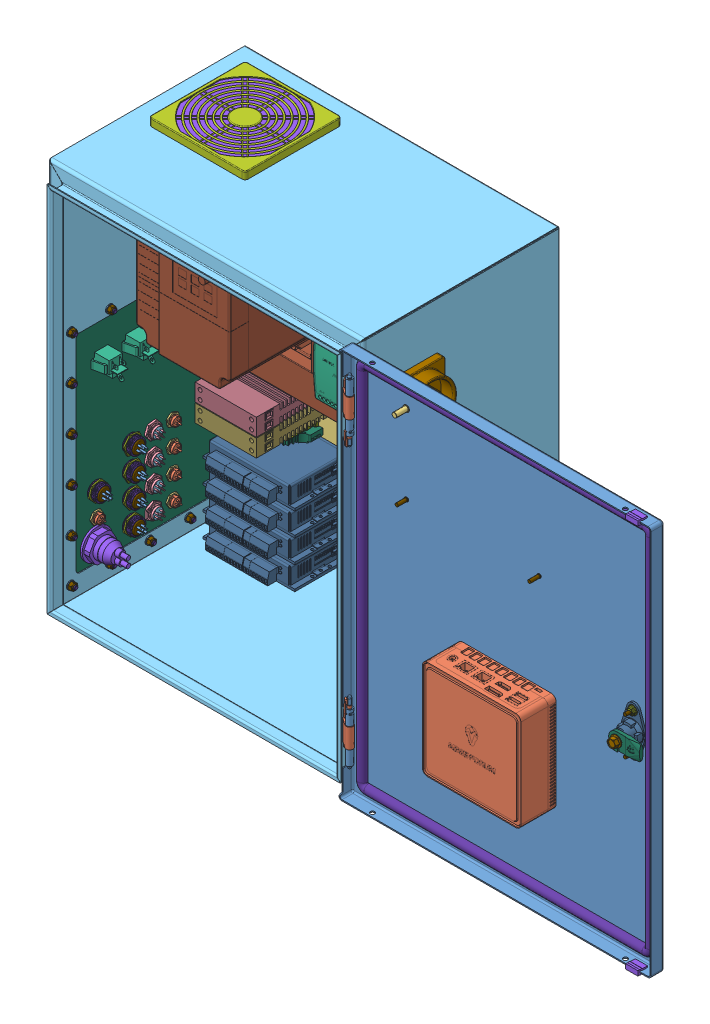
SolidWorks assembly CNC Control Panel, configuration Door Open. Lengths in mm. (continued)
Components (placement in the parent): (continued)
- CL57Y Stepper Driver-15: CL57Y Stepper Driver [Default] at (-96.34 -163.14 63.8842) x (0 0 1) z (0 1 0) size (89.31 118 24.2)
- CL57Y Stepper Driver-16: CL57Y Stepper Driver [Default] at (-96.34 -133.14 63.8842) x (0 0 1) z (0 1 0) size (89.31 118 24.2)
- 7641K526_MODULAR DIN RAIL-MOUNT TERMINAL BLOCK-3: 7641K526_MODULAR DIN RAIL-MOUNT TERMINAL BLOCK [7641K526] at (18.04 186.09 73.9842) x (1 0 0) z (0 -1 0) size (8.38 46.95 44.65)
- 7641K526_MODULAR DIN RAIL-MOUNT TERMINAL BLOCK-4: 7641K526_MODULAR DIN RAIL-MOUNT TERMINAL BLOCK [7641K526] at (26.24 186.09 73.9842) x (1 0 0) z (0 -1 0) size (8.38 46.95 44.65)
- 7641K526_MODULAR DIN RAIL-MOUNT TERMINAL BLOCK-5: 7641K526_MODULAR DIN RAIL-MOUNT TERMINAL BLOCK [7641K526] at (34.44 186.09 73.9842) x (1 0 0) z (0 -1 0) size (8.38 46.95 44.65)
- 7641K526_MODULAR DIN RAIL-MOUNT TERMINAL BLOCK-6: 7641K526_MODULAR DIN RAIL-MOUNT TERMINAL BLOCK [7641K526] at (42.64 186.09 73.9842) x (1 0 0) z (0 -1 0) size (8.38 46.95 44.65)
- 7641K526_MODULAR DIN RAIL-MOUNT TERMINAL BLOCK-7: 7641K526_MODULAR DIN RAIL-MOUNT TERMINAL BLOCK [7641K526] at (50.84 186.09 73.9842) x (1 0 0) z (0 -1 0) size (8.38 46.95 44.65)
- 7641K526_MODULAR DIN RAIL-MOUNT TERMINAL BLOCK-8: 7641K526_MODULAR DIN RAIL-MOUNT TERMINAL BLOCK [7641K526] at (59.04 186.09 73.9842) x (1 0 0) z (0 -1 0) size (8.38 46.95 44.65)
- 7641K526_MODULAR DIN RAIL-MOUNT TERMINAL BLOCK-9: 7641K526_MODULAR DIN RAIL-MOUNT TERMINAL BLOCK [7641K526] at (67.24 186.09 73.9842) x (1 0 0) z (0 -1 0) size (8.38 46.95 44.65)
- 7641K526_MODULAR DIN RAIL-MOUNT TERMINAL BLOCK-10: 7641K526_MODULAR DIN RAIL-MOUNT TERMINAL BLOCK [7641K526] at (75.44 186.09 73.9842) x (1 0 0) z (0 -1 0) size (8.38 46.95 44.65)
- 7641K526_MODULAR DIN RAIL-MOUNT TERMINAL BLOCK-11: 7641K526_MODULAR DIN RAIL-MOUNT TERMINAL BLOCK [7641K526] at (83.64 186.09 73.9842) x (1 0 0) z (0 -1 0) size (8.38 46.95 44.65)
- AD-SSR630-22-DCZ-1: AD-SSR630-22-DCZ [Default] at (-103.1569 -64.468 28.4042) size (101.09 22.35 96.52)
- AD-SSR210-22-DCZ-1: AD-SSR210-22-DCZ [Default] at (-103.1569 -41.116 28.4042) size (101.09 22.35 96.52)
- 7641K924_MODULAR DIN RAIL-MOUNT TERMINAL BLOCK-2: 7641K924_MODULAR DIN RAIL-MOUNT TERMINAL BLOCK [7641K924] at (-105.067 -86.744 73.9842) x (0 1 0) z (1 0 0) size (7 46.95 44.65)
- 7641K924_MODULAR DIN RAIL-MOUNT TERMINAL BLOCK-3: 7641K924_MODULAR DIN RAIL-MOUNT TERMINAL BLOCK [7641K924] at (-105.067 -91.844 73.9842) x (0 1 0) z (1 0 0) size (7 46.95 44.65)
- 7641K924_MODULAR DIN RAIL-MOUNT TERMINAL BLOCK-4: 7641K924_MODULAR DIN RAIL-MOUNT TERMINAL BLOCK [7641K924] at (-105.067 -96.944 73.9842) x (0 1 0) z (1 0 0) size (7 46.95 44.65)
Mates (geometry in assembly coordinates):
- Coincident1: coincident: plane of YuCo YC-20X16X10-UL-1/87934540-1/87934343_default-1 through (0 0 0) normal (0 0 1); plane of assembly through (0 0 0) normal (0 0 1)
- Coincident2: coincident: plane of YuCo YC-20X16X10-UL-1/87934540-1/87934343_default-1 through (0 0 0) normal (-1 0 0); plane of assembly through (0 0 0) normal (1 0 0)
- Coincident3: coincident: plane of YuCo YC-20X16X10-UL-1/87934540-1/87934343_default-1 through (0 0 0) normal (0 -1 0); plane of assembly through (0 0 0) normal (0 1 0)
- Coincident4: coincident: plane of YuCo YC-20X16X10-UL-1/64403004-1 through (180.34 231.14 25.9842) normal (0 0 1); plane of SCN-1000-48-1/SCN-1000-48 PSU-1 through (170.34 206.14 25.9842) normal (0 0 -1)
- Coincident5: coincident: plane of YuCo YC-20X16X10-UL-1/64403004-1 through (180.34 231.14 25.9842) normal (0 0 1); plane of GT-2R2G-2 (220V) Huanyang VFD-1 through (-99.5316 125.3316 25.9842) normal (0 0 -1)
- Coincident9: coincident: plane of YuCo YC-20X16X10-UL-1/64403004-1 through (180.34 231.14 25.9842) normal (0 0 1); plane of CL57Y Stepper Driver-1 through (-155.34 -220.14 25.9842) normal (0 0 -1)
- Coincident26: coincident: plane of YuCo YC-20X16X10-UL-1/64403004-1 through (180.34 231.14 25.9842) normal (0 0 1); plane of 7578K262_SLOTTED WIRE DUCT WITH SNAP-ON COVER-1 through (-30.4441 -872.2624 25.9842) normal (0 0 -1)
- Distance7: distance = 5 mm: plane of 7578K262_SLOTTED WIRE DUCT WITH SNAP-ON COVER-1 through (-32.0316 -872.2624 27.5717) normal (-1 0 0); plane of GT-2R2G-2 (220V) Huanyang VFD-1 through (-37.0316 37.8316 185.9842) normal (1 0 0)
- Distance8: distance = 40 mm: plane of GT-2R2G-2 (220V) Huanyang VFD-1 through (-162.0316 212.8316 185.9842) normal (0 1 0); plane of YuCo YC-20X16X10-UL-1/87934540-1/87934343_default-1 through (2743.2 252.8316 250.4186) normal (0 -1 0)
- Distance9: distance = 40 mm: plane of GT-2R2G-2 (220V) Huanyang VFD-1 through (-162.0316 37.8316 185.9842) normal (-1 0 0); plane of YuCo YC-20X16X10-UL-1/87934540-1/87934343_default-1 through (-202.0316 2794 250.4186) normal (1 0 0)
- Distance10: distance = 10 mm: plane of YuCo YC-20X16X10-UL-1/64403004-1 through (180.34 -231.14 25.9842) normal (1 0 0); plane of SCN-1000-48-1/SCN-1000-48 PSU-1 through (170.34 60.64 91.9842) normal (1 0 0)
- Coincident34: coincident: plane of ALIM MEAN WELL MDR-2 through (53.44 62.14 33.4842) normal (0 0 -1); plane of 8961K150_DIN RAIL (1)-1 through (10.44 91.14 33.4842) normal (0 0 1)
- Coincident35: coincident: plane of ALIM MEAN WELL MDR-1 through (95.44 62.14 33.4842) normal (0 0 -1); plane of 8961K150_DIN RAIL (1)-1 through (10.44 91.14 33.4842) normal (0 0 1)
- Coincident36: coincident: plane of ALIM MEAN WELL MDR-1 through (95.44 91.14 31.9842) normal (0 -1 0); plane of 8961K150_DIN RAIL (1)-1 through (10.44 91.14 33.4842) normal (0 1 0)
- Coincident37: coincident: plane of ALIM MEAN WELL MDR-2 through (53.44 91.14 31.9842) normal (0 -1 0); plane of 8961K150_DIN RAIL (1)-1 through (10.44 91.14 33.4842) normal (0 1 0)
- Distance12: distance = 2 mm: plane of ALIM MEAN WELL MDR-1 through (55.44 73.64 129.4842) normal (-1 0 0); plane of ALIM MEAN WELL MDR-2 through (53.44 73.64 129.4842) normal (1 0 0)
- Distance13: distance = 3 mm: plane of ALIM MEAN WELL MDR-2 through (13.44 73.64 129.4842) normal (-1 0 0); plane of 8961K150_DIN RAIL (1)-1 through (10.44 59.64 31.9842) normal (-1 0 0)
- Coincident40: coincident: plane of YuCo YC-20X16X10-UL-1/64403004-1 through (180.34 231.14 25.9842) normal (0 0 1); plane of 8961K150_DIN RAIL (1)-1 through (10.44 86.14 25.9842) normal (0 0 -1)
- Distance14: distance = 140 mm: plane of 8961K150_DIN RAIL (1)-1 through (10.44 91.14 33.4842) normal (0 1 0); plane of YuCo YC-20X16X10-UL-1/64403004-1 through (180.34 231.14 25.9842) normal (0 1 0)
- Coincident42: coincident: plane of YuCo YC-20X16X10-UL-1/64403004-1 through (180.34 231.14 25.9842) normal (0 0 1); plane of 7578K262_SLOTTED WIRE DUCT WITH SNAP-ON COVER-3 through (832.04 -21.5525 25.9842) normal (0 0 -1)
- Coincident43: coincident: plane of 7578K262_SLOTTED WIRE DUCT WITH SNAP-ON COVER-1 through (-12.0928 16.7376 25.9842) normal (0 -1 0); plane of 7578K262_SLOTTED WIRE DUCT WITH SNAP-ON COVER-3 through (832.04 16.7376 27.5717) normal (0 1 0)
- Distance16: distance = 25 mm: plane of SCN-1000-48-1/SCN-1000-48 PSU-1 through (170.34 206.14 157.9842) normal (0 1 0); plane of YuCo YC-20X16X10-UL-1/64403004-1 through (180.34 231.14 25.9842) normal (0 1 0)
- Coincident52: coincident: plane of ALIM MEAN WELL MDR-1 through (95.44 73.64 129.4842) normal (1 0 0); plane of 7578K262_SLOTTED WIRE DUCT WITH SNAP-ON COVER-3 through (95.44 -3.2012 25.9842) normal (1 0 0)
- Distance21: distance = 3 mm: plane of SCN-1000-48-1/SCN-1000-48 PSU-1 through (102.34 60.64 91.9842) normal (-1 0 0); plane of 8961K150_DIN RAIL (1)-1 through (99.34 73.64 25.9842) normal (1 0 0)
- Coincident54: coincident: plane of YuCo YC-20X16X10-UL-1/87934540-1/87934343_default-1 through (202.0316 -2794 250.4186) normal (-1 0 0); plane of 120mm Fan-1 through (202.0316 -179 160) normal (1 0 0)
- Coincident57: coincident: plane of YuCo YC-20X16X10-UL-1/87934540-1/87934343_default-1 through (203.2 -2794 250.4186) normal (1 0 0); plane of 120mm Filter-1/Cover-1 through (203.2 -179 160) normal (-1 0 0)
- Distance25: distance = 8 mm: plane of CL57Y Stepper Driver-1 through (-96.34 -223.14 63.8842) normal (0 -1 0); plane of YuCo YC-20X16X10-UL-1/64403004-1 through (180.34 -231.14 25.9842) normal (0 -1 0)
- Distance26: distance = 25 mm: plane of CL57Y Stepper Driver-1 through (-155.34 -220.14 25.9842) normal (-1 0 0); plane of YuCo YC-20X16X10-UL-1/64403004-1 through (-180.34 -231.14 25.9842) normal (-1 0 0)
- Coincident63: coincident: plane of YuCo YC-20X16X10-UL-1/64403004-1 through (180.34 231.14 25.9842) normal (0 0 1); plane of 8961K150_DIN RAIL (1)-2 through (-115.34 -104.14 25.9842) normal (0 0 -1)
- Distance31: distance = 60 mm: plane of 8961K150_DIN RAIL (1)-2 through (-120.34 -104.14 33.4842) normal (-1 0 0); plane of YuCo YC-20X16X10-UL-1/64403004-1 through (-180.34 -231.14 25.9842) normal (-1 0 0)
- Distance32: distance = 127 mm: plane of 8961K150_DIN RAIL (1)-2 through (-88.84 -104.14 31.9842) normal (0 -1 0); plane of YuCo YC-20X16X10-UL-1/64403004-1 through (180.34 -231.14 25.9842) normal (0 -1 0)
- Coincident92: coincident: plane of YuCo YC-20X16X10-UL-1/64403004-1 through (180.34 231.14 25.9842) normal (0 0 1); plane of 8961K150_DIN RAIL (1)-3 through (-31.66 196.14 25.9842) normal (0 0 -1)
- Distance38: distance = 30 mm: plane of 8961K150_DIN RAIL (1)-3 through (-31.66 201.14 33.4842) normal (0 1 0); plane of YuCo YC-20X16X10-UL-1/64403004-1 through (180.34 231.14 25.9842) normal (0 1 0)
- Distance39: distance = 85 mm: plane of YuCo YC-20X16X10-UL-1/64403004-1 through (180.34 -231.14 25.9842) normal (1 0 0); plane of 8961K150_DIN RAIL (1)-3 through (95.34 183.64 25.9842) normal (1 0 0)
- Coincident95: coincident: plane of YuCo YC-20X16X10-UL-1/87934540-1/87934343_default-1 through (203.2 -2794 250.4186) normal (1 0 0); plane of ALLEN-BRADLEY_194E-E25-1753-6N-1 through (203.2 159 190) normal (-1 0 0)
- Coincident99: coincident: plane of 8961K150_DIN RAIL (1)-3 through (-31.66 201.14 33.4842) normal (0 0 1); plane of Lovato Electric FB01F1P-4 through (-12.66 165.5766 33.4842) normal (0 0 -1)
- Coincident100: coincident: line of 8961K150_DIN RAIL (1)-3 through (-31.66 201.14 33.4842) axis (1 0 0); plane of Lovato Electric FB01F1P-4 through (-12.66 201.14 33.4842) normal (0 -1 0)
- Distance43: distance = 208 mm: plane of 7578K262_SLOTTED WIRE DUCT WITH SNAP-ON COVER-3 through (832.04 -23.14 27.5717) normal (0 -1 0); line of YuCo YC-20X16X10-UL-1/64403004-1 through (160.3756 -231.14 25.9842) axis (-1 0 0)
- Coincident102: coincident: plane of 8961K150_DIN RAIL (1)-3 through (-31.66 201.14 33.4842) normal (0 0 1); plane of Lovato Electric FB01F1P-5 through (5.34 165.5766 33.4842) normal (0 0 -1)
- Coincident103: coincident: line of 8961K150_DIN RAIL (1)-3 through (-31.66 201.14 33.4842) axis (1 0 0); plane of Lovato Electric FB01F1P-5 through (5.34 201.14 33.4842) normal (0 -1 0)
- Distance44: distance = 1.5 mm: plane of Lovato Electric FB01F1P-4 through (-30.16 183.7092 53.8516) normal (-1 0 0); line of 8961K150_DIN RAIL (1)-3 through (-31.66 171.64 26.9842) axis (0 1 0)
- Distance45: distance = 0.5 mm: plane of Lovato Electric FB01F1P-5 through (-12.16 183.7092 53.8516) normal (-1 0 0); plane of Lovato Electric FB01F1P-4 through (-12.66 183.7092 53.8516) normal (1 0 0)
- Coincident115: coincident: plane of 8961K150_DIN RAIL (1)-3 through (-31.66 201.14 33.4842) normal (0 0 1); plane of 7641K526_MODULAR DIN RAIL-MOUNT TERMINAL BLOCK-2 through (5.84 188.24 33.4842) normal (0 0 -1)
- Coincident116: coincident: line of 8961K150_DIN RAIL (1)-3 through (-31.66 201.14 33.4842) axis (1 0 0); plane of 7641K526_MODULAR DIN RAIL-MOUNT TERMINAL BLOCK-2 through (5.84 201.14 37.0342) normal (0 -1 0)
- Distance47: distance = 0.5 mm: plane of Lovato Electric FB01F1P-5 through (5.34 183.7092 53.8516) normal (1 0 0); plane of 7641K526_MODULAR DIN RAIL-MOUNT TERMINAL BLOCK-2 through (5.84 162.54 27.5342) normal (-1 0 0)
- Coincident118: coincident: plane of 8961K150_DIN RAIL (1)-3 through (-31.66 166.14 33.4842) normal (0 0 1); plane of 7641K350_MODULAR DIN RAIL-MOUNT TERMINAL BLOCK-1 through (92.64 201.14 33.4842) normal (0 0 -1)
- Coincident119: coincident: line of 8961K150_DIN RAIL (1)-3 through (-31.66 201.14 33.4842) axis (1 0 0); line of 7641K350_MODULAR DIN RAIL-MOUNT TERMINAL BLOCK-1 through (87.64 201.14 33.4842) axis (1 0 0)
- Coincident120: coincident: plane of 7641K526_MODULAR DIN RAIL-MOUNT TERMINAL BLOCK-11 through (87.64 162.54 27.5342) normal (1 0 0); plane of 7641K350_MODULAR DIN RAIL-MOUNT TERMINAL BLOCK-1 through (87.64 183.4399 45.1047) normal (-1 0 0)
- Coincident129: coincident: plane of 8961K150_DIN RAIL (1)-2 through (-120.34 -104.14 33.4842) normal (0 0 1); plane of AD-SSR210-22-DCZ-1 through (-103.1569 -41.116 33.4842) normal (0 0 -1)
- Coincident130: coincident: plane of 8961K150_DIN RAIL (1)-2 through (-120.34 -104.14 33.4842) normal (0 0 1); plane of AD-SSR630-22-DCZ-1 through (-103.1569 -64.468 33.4842) normal (0 0 -1)
- Coincident133: coincident: line of 8961K150_DIN RAIL (1)-2 through (-120.34 -104.14 33.4842) axis (0 1 0); plane of AD-SSR210-22-DCZ-1 through (-120.34 -1.746 30.0984) normal (1 0 0)
- Coincident134: coincident: line of 8961K150_DIN RAIL (1)-2 through (-120.34 -104.14 33.4842) axis (0 1 0); plane of AD-SSR630-22-DCZ-1 through (-120.34 -25.098 30.0984) normal (1 0 0)
- Distance52: distance = 2 mm: plane of AD-SSR210-22-DCZ-1 through (-103.1569 -29.94 36.0242) normal (0 1 0); line of 8961K150_DIN RAIL (1)-2 through (-90.84 -27.94 26.9842) axis (-1 0 0)
- Distance53: distance = 1 mm: plane of AD-SSR210-22-DCZ-1 through (-103.1569 -52.292 96.9842) normal (0 -1 0); plane of AD-SSR630-22-DCZ-1 through (-103.1569 -53.292 96.9842) normal (0 1 0)
- Coincident138: coincident: plane of 8961K150_DIN RAIL (1)-2 through (-85.34 -104.14 33.4842) normal (0 0 1); plane of 7641K924_MODULAR DIN RAIL-MOUNT TERMINAL BLOCK-1 through (-108.215 -76.644 33.4842) normal (0 0 -1)
- Coincident139: coincident: plane of 8961K150_DIN RAIL (1)-2 through (-85.34 -104.14 33.4842) normal (1 0 0); plane of 7641K924_MODULAR DIN RAIL-MOUNT TERMINAL BLOCK-1 through (-85.34 -76.644 32.4811) normal (-1 0 0)
- Distance54: distance = 1 mm: plane of 7641K924_MODULAR DIN RAIL-MOUNT TERMINAL BLOCK-1 through (-81.565 -76.644 27.5342) normal (0 1 0); plane of AD-SSR630-22-DCZ-1 through (-103.1569 -75.644 96.9842) normal (0 -1 0)
- Coincident146: coincident: plane of 8961K150_DIN RAIL (1)-2 through (-120.34 -104.14 33.4842) normal (0 0 1); plane of 7641K350_MODULAR DIN RAIL-MOUNT TERMINAL BLOCK-2 through (-84.94 -101.944 33.4842) normal (0 0 -1)
- Coincident147: coincident: plane of 7641K924_MODULAR DIN RAIL-MOUNT TERMINAL BLOCK-4 through (-81.565 -96.944 27.5342) normal (0 -1 0); plane of 7641K350_MODULAR DIN RAIL-MOUNT TERMINAL BLOCK-2 through (-102.6401 -96.944 45.1047) normal (0 1 0)
- Coincident148: coincident: line of 8961K150_DIN RAIL (1)-2 through (-120.34 -104.14 33.4842) axis (0 1 0); line of 7641K350_MODULAR DIN RAIL-MOUNT TERMINAL BLOCK-2 through (-120.34 -98.944 33.4842) axis (0 -1 0)
- Concentric3: concentric: cylinder of YuCo YC-20X16X10-UL-1/87934540-1/87934343_default-1 through (-203.201 -179 160) axis (1 0 0) radius 57.5; cylinder of 120mm Fan-1 through (164.0316 -179 160) axis (1 0 0) radius 58
- Concentric4: concentric: cylinder of YuCo YC-20X16X10-UL-1/87934540-1/87934343_default-1 through (-203.201 -231.5 212.5) axis (1 0 0) radius 2.5; cylinder of 120mm Fan-1 through (202.0316 -231.5 212.5) axis (-1 0 0) radius 2.15
- Concentric5: concentric: cylinder of YuCo YC-20X16X10-UL-1/87934540-1/87934343_default-1 through (-203.201 -179 160) axis (1 0 0) radius 57.5; circle of 120mm Filter-1/Cover-1
- Concentric6: concentric: cylinder of YuCo YC-20X16X10-UL-1/87934540-1/87934343_default-1 through (-203.201 -231.5 212.5) axis (1 0 0) radius 2.5; cylinder of 120mm Filter-1/Base-1 through (203.2 -231.5 212.5) axis (1 0 0) radius 2.5
- Coincident152: coincident: plane of YuCo YC-20X16X10-UL-1/87934540-1/87934343_default-1 through (2743.2 254 250.4186) normal (0 1 0); plane of 120mm Filter-2/Cover-1 through (-113.2 254 90) normal (0 -1 0)
- Concentric7: concentric: cylinder of YuCo YC-20X16X10-UL-1/87934540-1/87934343_default-1 through (-113.2 -254.001 90) axis (0 1 0) radius 57.5; circle of 120mm Filter-2/Cover-1
- Concentric8: concentric: cylinder of YuCo YC-20X16X10-UL-1/87934540-1/87934343_default-1 through (-165.7 -254.001 37.5) axis (0 1 0) radius 2.5; cylinder of 120mm Filter-2/Base-1 through (-165.7 254 37.5) axis (0 1 0) radius 2.5
- Coincident156: coincident: plane of YuCo YC-20X16X10-UL-1/87934540-1/87934343_default-1 through (-203.2 2794 250.4186) normal (-1 0 0); plane of Gland Plate Assembly-1/Controller Gland Plate-1 through (-203.2 -234 25) normal (1 0 0)
- Distance58: distance = 15 mm: plane of YuCo YC-20X16X10-UL-1/87934540-1/87934343_default-1 through (203.2 254 0) normal (0 0 -1); plane of Gland Plate Assembly-1/Controller Gland Plate-1 through (-205.2 -234 15) normal (0 0 -1)
- Distance59: distance = 10 mm: plane of Gland Plate Assembly-1/Controller Gland Plate-1 through (-205.2 -244 25) normal (0 -1 0); plane of YuCo YC-20X16X10-UL-1/87934540-1/87934343_default-1 through (-2743.2 -254 250.4186) normal (0 -1 0)
- Concentric13: concentric: cylinder of Gland Plate Assembly-1/Controller Gland Plate-1 through (-203.2 47.4142 23.5858) axis (-1 0 0) radius 2.525; cylinder of M5 Bolt Nut Washer Assembly-1/Trimcraft M5 BSC-1 through (-194.3 47.4142 23.5858) axis (1 0 0) radius 2.5
- Coincident163: coincident: plane of Gland Plate Assembly-1/Controller Gland Plate-1 through (-205.2 -234 25) normal (-1 0 0); plane of M5 Bolt Nut Washer Assembly-1/Trimcraft M5 Washer-2 through (-205.2 47.4142 23.5858) normal (1 0 0)
- Coincident164: coincident: plane of YuCo YC-20X16X10-UL-1/87934540-1/87934343_default-1 through (-202.0316 2794 250.4186) normal (1 0 0); plane of M5 Bolt Nut Washer Assembly-1/Trimcraft M5 Washer-1 through (-202.0316 47.4142 23.5858) normal (-1 0 0)
- Coincident165: coincident: plane of Gland Plate Assembly-1/Controller Gland Plate-1 through (-205.2 -234 25) normal (-1 0 0); plane of M5 Bolt Nut Washer Assembly-2/Trimcraft M5 Washer-2 through (-205.2 48 74) normal (1 0 0)
- Coincident166: coincident: plane of YuCo YC-20X16X10-UL-1/87934540-1/87934343_default-1 through (-202.0316 2794 250.4186) normal (1 0 0); plane of M5 Bolt Nut Washer Assembly-2/Trimcraft M5 Washer-1 through (-202.0316 48 74) normal (-1 0 0)
- Concentric14: concentric: cylinder of Gland Plate Assembly-1/Controller Gland Plate-1 through (-203.2 48 74) axis (-1 0 0) radius 2.525; cylinder of M5 Bolt Nut Washer Assembly-2/Trimcraft M5 BSC-1 through (-194.3 48 74) axis (1 0 0) radius 2.5
- Coincident167: coincident: plane of Gland Plate Assembly-1/Controller Gland Plate-1 through (-205.2 -234 25) normal (-1 0 0); plane of M5 Bolt Nut Washer Assembly-3/Trimcraft M5 Washer-2 through (-205.2 48 125) normal (1 0 0)
- Coincident168: coincident: plane of YuCo YC-20X16X10-UL-1/87934540-1/87934343_default-1 through (-202.0316 2794 250.4186) normal (1 0 0); plane of M5 Bolt Nut Washer Assembly-3/Trimcraft M5 Washer-1 through (-202.0316 48 125) normal (-1 0 0)
- Concentric15: concentric: cylinder of Gland Plate Assembly-1/Controller Gland Plate-1 through (-203.2 48 125) axis (-1 0 0) radius 2.525; cylinder of M5 Bolt Nut Washer Assembly-3/Trimcraft M5 BSC-1 through (-194.3 48 125) axis (1 0 0) radius 2.5
- Coincident169: coincident: plane of Gland Plate Assembly-1/Controller Gland Plate-1 through (-205.2 -234 25) normal (-1 0 0); plane of M5 Bolt Nut Washer Assembly-4/Trimcraft M5 Washer-2 through (-205.2 48 176) normal (1 0 0)
- Coincident170: coincident: plane of YuCo YC-20X16X10-UL-1/87934540-1/87934343_default-1 through (-202.0316 2794 250.4186) normal (1 0 0); plane of M5 Bolt Nut Washer Assembly-4/Trimcraft M5 Washer-1 through (-202.0316 48 176) normal (-1 0 0)
- Concentric16: concentric: cylinder of Gland Plate Assembly-1/Controller Gland Plate-1 through (-203.2 48 176) axis (-1 0 0) radius 2.525; cylinder of M5 Bolt Nut Washer Assembly-4/Trimcraft M5 BSC-1 through (-194.3 48 176) axis (1 0 0) radius 2.5
- Coincident171: coincident: plane of Gland Plate Assembly-1/Controller Gland Plate-1 through (-205.2 -234 25) normal (-1 0 0); plane of M5 Bolt Nut Washer Assembly-5/Trimcraft M5 Washer-2 through (-205.2 47.4142 226.4142) normal (1 0 0)
- Coincident172: coincident: plane of YuCo YC-20X16X10-UL-1/87934540-1/87934343_default-1 through (-202.0316 2794 250.4186) normal (1 0 0); plane of M5 Bolt Nut Washer Assembly-5/Trimcraft M5 Washer-1 through (-202.0316 47.4142 226.4142) normal (-1 0 0)
- Concentric17: concentric: cylinder of Gland Plate Assembly-1/Controller Gland Plate-1 through (-203.2 47.4142 226.4142) axis (-1 0 0) radius 2.525; cylinder of M5 Bolt Nut Washer Assembly-5/Trimcraft M5 BSC-1 through (-194.3 47.4142 226.4142) axis (1 0 0) radius 2.5
- Coincident173: coincident: plane of Gland Plate Assembly-1/Controller Gland Plate-1 through (-205.2 -234 25) normal (-1 0 0); plane of M5 Bolt Nut Washer Assembly-6/Trimcraft M5 Washer-2 through (-205.2 -8.8 227) normal (1 0 0)
- Coincident174: coincident: plane of YuCo YC-20X16X10-UL-1/87934540-1/87934343_default-1 through (-202.0316 2794 250.4186) normal (1 0 0); plane of M5 Bolt Nut Washer Assembly-6/Trimcraft M5 Washer-1 through (-202.0316 -8.8 227) normal (-1 0 0)
- Concentric18: concentric: cylinder of Gland Plate Assembly-1/Controller Gland Plate-1 through (-203.2 -8.8 227) axis (-1 0 0) radius 2.525; cylinder of M5 Bolt Nut Washer Assembly-6/Trimcraft M5 BSC-1 through (-194.3 -8.8 227) axis (1 0 0) radius 2.5
- Coincident175: coincident: plane of Gland Plate Assembly-1/Controller Gland Plate-1 through (-205.2 -234 25) normal (-1 0 0); plane of M5 Bolt Nut Washer Assembly-7/Trimcraft M5 Washer-2 through (-205.2 -65.6 227) normal (1 0 0)
- Coincident176: coincident: plane of YuCo YC-20X16X10-UL-1/87934540-1/87934343_default-1 through (-202.0316 2794 250.4186) normal (1 0 0); plane of M5 Bolt Nut Washer Assembly-7/Trimcraft M5 Washer-1 through (-202.0316 -65.6 227) normal (-1 0 0)
- Concentric19: concentric: cylinder of Gland Plate Assembly-1/Controller Gland Plate-1 through (-203.2 -65.6 227) axis (-1 0 0) radius 2.525; cylinder of M5 Bolt Nut Washer Assembly-7/Trimcraft M5 BSC-1 through (-194.3 -65.6 227) axis (1 0 0) radius 2.5
- Coincident177: coincident: plane of Gland Plate Assembly-1/Controller Gland Plate-1 through (-205.2 -234 25) normal (-1 0 0); plane of M5 Bolt Nut Washer Assembly-8/Trimcraft M5 Washer-2 through (-205.2 -122.4 227) normal (1 0 0)
- Coincident178: coincident: plane of YuCo YC-20X16X10-UL-1/87934540-1/87934343_default-1 through (-202.0316 2794 250.4186) normal (1 0 0); plane of M5 Bolt Nut Washer Assembly-8/Trimcraft M5 Washer-1 through (-202.0316 -122.4 227) normal (-1 0 0)
- Concentric20: concentric: cylinder of Gland Plate Assembly-1/Controller Gland Plate-1 through (-203.2 -122.4 227) axis (-1 0 0) radius 2.525; cylinder of M5 Bolt Nut Washer Assembly-8/Trimcraft M5 BSC-1 through (-194.3 -122.4 227) axis (1 0 0) radius 2.5
- Coincident179: coincident: plane of Gland Plate Assembly-1/Controller Gland Plate-1 through (-205.2 -234 25) normal (-1 0 0); plane of M5 Bolt Nut Washer Assembly-9/Trimcraft M5 Washer-2 through (-205.2 -179.2 227) normal (1 0 0)
- Coincident180: coincident: plane of YuCo YC-20X16X10-UL-1/87934540-1/87934343_default-1 through (-202.0316 2794 250.4186) normal (1 0 0); plane of M5 Bolt Nut Washer Assembly-9/Trimcraft M5 Washer-1 through (-202.0316 -179.2 227) normal (-1 0 0)
- Concentric21: concentric: cylinder of Gland Plate Assembly-1/Controller Gland Plate-1 through (-203.2 -179.2 227) axis (-1 0 0) radius 2.525; cylinder of M5 Bolt Nut Washer Assembly-9/Trimcraft M5 BSC-1 through (-194.3 -179.2 227) axis (1 0 0) radius 2.5
- Coincident181: coincident: plane of Gland Plate Assembly-1/Controller Gland Plate-1 through (-205.2 -234 25) normal (-1 0 0); plane of M5 Bolt Nut Washer Assembly-10/Trimcraft M5 Washer-2 through (-205.2 -235.4142 226.4142) normal (1 0 0)
- Coincident182: coincident: plane of YuCo YC-20X16X10-UL-1/87934540-1/87934343_default-1 through (-202.0316 2794 250.4186) normal (1 0 0); plane of M5 Bolt Nut Washer Assembly-10/Trimcraft M5 Washer-1 through (-202.0316 -235.4142 226.4142) normal (-1 0 0)
- Concentric22: concentric: cylinder of Gland Plate Assembly-1/Controller Gland Plate-1 through (-203.2 -235.4142 226.4142) axis (-1 0 0) radius 2.525; cylinder of M5 Bolt Nut Washer Assembly-10/Trimcraft M5 BSC-1 through (-194.3 -235.4142 226.4142) axis (1 0 0) radius 2.5
- Coincident183: coincident: plane of Gland Plate Assembly-1/Controller Gland Plate-1 through (-205.2 -234 25) normal (-1 0 0); plane of M5 Bolt Nut Washer Assembly-11/Trimcraft M5 Washer-2 through (-205.2 -236 176) normal (1 0 0)
- Coincident184: coincident: plane of YuCo YC-20X16X10-UL-1/87934540-1/87934343_default-1 through (-202.0316 2794 250.4186) normal (1 0 0); plane of M5 Bolt Nut Washer Assembly-11/Trimcraft M5 Washer-1 through (-202.0316 -236 176) normal (-1 0 0)
- Concentric23: concentric: cylinder of Gland Plate Assembly-1/Controller Gland Plate-1 through (-203.2 -236 176) axis (-1 0 0) radius 2.525; cylinder of M5 Bolt Nut Washer Assembly-11/Trimcraft M5 BSC-1 through (-194.3 -236 176) axis (1 0 0) radius 2.5
- Coincident185: coincident: plane of Gland Plate Assembly-1/Controller Gland Plate-1 through (-205.2 -234 25) normal (-1 0 0); plane of M5 Bolt Nut Washer Assembly-12/Trimcraft M5 Washer-2 through (-205.2 -236 125) normal (1 0 0)
- Coincident186: coincident: plane of YuCo YC-20X16X10-UL-1/87934540-1/87934343_default-1 through (-202.0316 2794 250.4186) normal (1 0 0); plane of M5 Bolt Nut Washer Assembly-12/Trimcraft M5 Washer-1 through (-202.0316 -236 125) normal (-1 0 0)
- Concentric24: concentric: cylinder of Gland Plate Assembly-1/Controller Gland Plate-1 through (-203.2 -236 125) axis (-1 0 0) radius 2.525; cylinder of M5 Bolt Nut Washer Assembly-12/Trimcraft M5 BSC-1 through (-194.3 -236 125) axis (1 0 0) radius 2.5
- Coincident187: coincident: plane of Gland Plate Assembly-1/Controller Gland Plate-1 through (-205.2 -234 25) normal (-1 0 0); plane of M5 Bolt Nut Washer Assembly-13/Trimcraft M5 Washer-2 through (-205.2 -236 74) normal (1 0 0)
- Coincident188: coincident: plane of YuCo YC-20X16X10-UL-1/87934540-1/87934343_default-1 through (-202.0316 2794 250.4186) normal (1 0 0); plane of M5 Bolt Nut Washer Assembly-13/Trimcraft M5 Washer-1 through (-202.0316 -236 74) normal (-1 0 0)
- Concentric25: concentric: cylinder of Gland Plate Assembly-1/Controller Gland Plate-1 through (-203.2 -236 74) axis (-1 0 0) radius 2.525; cylinder of M5 Bolt Nut Washer Assembly-13/Trimcraft M5 BSC-1 through (-194.3 -236 74) axis (1 0 0) radius 2.5
- Coincident189: coincident: plane of Gland Plate Assembly-1/Controller Gland Plate-1 through (-205.2 -234 25) normal (-1 0 0); plane of M5 Bolt Nut Washer Assembly-14/Trimcraft M5 Washer-2 through (-205.2 -235.4142 23.5858) normal (1 0 0)
- Coincident190: coincident: plane of YuCo YC-20X16X10-UL-1/87934540-1/87934343_default-1 through (-202.0316 2794 250.4186) normal (1 0 0); plane of M5 Bolt Nut Washer Assembly-14/Trimcraft M5 Washer-1 through (-202.0316 -235.4142 23.5858) normal (-1 0 0)
- Concentric26: concentric: cylinder of Gland Plate Assembly-1/Controller Gland Plate-1 through (-203.2 -235.4142 23.5858) axis (-1 0 0) radius 2.525; cylinder of M5 Bolt Nut Washer Assembly-14/Trimcraft M5 BSC-1 through (-194.3 -235.4142 23.5858) axis (1 0 0) radius 2.5
- Coincident191: coincident: plane of Gland Plate Assembly-1/Controller Gland Plate-1 through (-205.2 -234 25) normal (-1 0 0); plane of M5 Bolt Nut Washer Assembly-15/Trimcraft M5 Washer-2 through (-205.2 -179.2 23) normal (1 0 0)
- Coincident192: coincident: plane of YuCo YC-20X16X10-UL-1/87934540-1/87934343_default-1 through (-202.0316 2794 250.4186) normal (1 0 0); plane of M5 Bolt Nut Washer Assembly-15/Trimcraft M5 Washer-1 through (-202.0316 -179.2 23) normal (-1 0 0)
- Concentric27: concentric: cylinder of Gland Plate Assembly-1/Controller Gland Plate-1 through (-203.2 -179.2 23) axis (-1 0 0) radius 2.525; cylinder of M5 Bolt Nut Washer Assembly-15/Trimcraft M5 BSC-1 through (-194.3 -179.2 23) axis (1 0 0) radius 2.5
- Coincident193: coincident: plane of Gland Plate Assembly-1/Controller Gland Plate-1 through (-205.2 -234 25) normal (-1 0 0); plane of M5 Bolt Nut Washer Assembly-16/Trimcraft M5 Washer-2 through (-205.2 -122.4 23) normal (1 0 0)
- Coincident194: coincident: plane of YuCo YC-20X16X10-UL-1/87934540-1/87934343_default-1 through (-202.0316 2794 250.4186) normal (1 0 0); plane of M5 Bolt Nut Washer Assembly-16/Trimcraft M5 Washer-1 through (-202.0316 -122.4 23) normal (-1 0 0)
- Concentric28: concentric: cylinder of Gland Plate Assembly-1/Controller Gland Plate-1 through (-203.2 -122.4 23) axis (-1 0 0) radius 2.525; cylinder of M5 Bolt Nut Washer Assembly-16/Trimcraft M5 BSC-1 through (-194.3 -122.4 23) axis (1 0 0) radius 2.5
- Coincident195: coincident: plane of Gland Plate Assembly-1/Controller Gland Plate-1 through (-205.2 -234 25) normal (-1 0 0); plane of M5 Bolt Nut Washer Assembly-17/Trimcraft M5 Washer-2 through (-205.2 -65.6 23) normal (1 0 0)
- Coincident196: coincident: plane of YuCo YC-20X16X10-UL-1/87934540-1/87934343_default-1 through (-202.0316 2794 250.4186) normal (1 0 0); plane of M5 Bolt Nut Washer Assembly-17/Trimcraft M5 Washer-1 through (-202.0316 -65.6 23) normal (-1 0 0)
- Concentric29: concentric: cylinder of Gland Plate Assembly-1/Controller Gland Plate-1 through (-203.2 -65.6 23) axis (-1 0 0) radius 2.525; cylinder of M5 Bolt Nut Washer Assembly-17/Trimcraft M5 BSC-1 through (-194.3 -65.6 23) axis (1 0 0) radius 2.5
- Coincident197: coincident: plane of Gland Plate Assembly-1/Controller Gland Plate-1 through (-205.2 -234 25) normal (-1 0 0); plane of M5 Bolt Nut Washer Assembly-18/Trimcraft M5 Washer-2 through (-205.2 -8.8 23) normal (1 0 0)
- Coincident198: coincident: plane of YuCo YC-20X16X10-UL-1/87934540-1/87934343_default-1 through (-202.0316 2794 250.4186) normal (1 0 0); plane of M5 Bolt Nut Washer Assembly-18/Trimcraft M5 Washer-1 through (-202.0316 -8.8 23) normal (-1 0 0)
- Concentric30: concentric: cylinder of Gland Plate Assembly-1/Controller Gland Plate-1 through (-203.2 -8.8 23) axis (-1 0 0) radius 2.525; cylinder of M5 Bolt Nut Washer Assembly-18/Trimcraft M5 BSC-1 through (-194.3 -8.8 23) axis (1 0 0) radius 2.5
- Coincident199: coincident: plane of AXBB-E-1 through (83.685 -104.215 36.9842) normal (0 0 -1); plane of CNCDrive_Parts_Mount-1 through (38.135 -161.215 36.9842) normal (0 0 1)
- Concentric31: concentric: cylinder of AXBB-E-1 through (-4.415 -216.215 39.9842) axis (0 0 -1) radius 2; cylinder of CNCDrive_Parts_Mount-1 through (-4.415 -216.215 25.9842) axis (0 0 1) radius 1.425
- Concentric32: concentric: cylinder of AXBB-E-1 through (80.685 -216.215 39.9842) axis (0 0 -1) radius 2; cylinder of CNCDrive_Parts_Mount-1 through (80.685 -216.215 25.9842) axis (0 0 1) radius 1.425
- Concentric33: concentric: cylinder of UCSB-1 through (-0.2243 -91.515 36.9842) axis (0 0 1) radius 1.75; cylinder of CNCDrive_Parts_Mount-1 through (-0.2243 -91.515 25.9842) axis (0 0 1) radius 1.425
- Concentric34: concentric: cylinder of UCSB-1 through (42.2757 -33.515 36.9842) axis (0 0 1) radius 1.75; cylinder of CNCDrive_Parts_Mount-1 through (42.2757 -33.515 25.9842) axis (0 0 1) radius 1.425
- Coincident200: coincident: plane of UCSB-1 through (25.6757 -62.365 36.9842) normal (0 0 -1); plane of CNCDrive_Parts_Mount-1 through (38.135 -161.215 36.9842) normal (0 0 1)
- Coincident201: coincident: plane of YuCo YC-20X16X10-UL-1/64403004-1 through (180.34 231.14 25.9842) normal (0 0 1); plane of CNCDrive_Parts_Mount-1 through (38.135 -161.215 25.9842) normal (0 0 -1)
- Distance60: distance = 10.5 mm: plane of CNCDrive_Parts_Mount-1 through (38.135 -220.64 25.9842) normal (0 -1 0); plane of YuCo YC-20X16X10-UL-1/64403004-1 through (180.34 -231.14 25.9842) normal (0 -1 0)
- Distance61: distance = 171.5 mm: plane of CNCDrive_Parts_Mount-1 through (-8.84 -161.215 25.9842) normal (-1 0 0); plane of YuCo YC-20X16X10-UL-1/64403004-1 through (-180.34 -231.14 25.9842) normal (-1 0 0)
- Coincident204: coincident: plane of YuCo YC-20X16X10-UL-1/87934540-1/87934343_default-1 through (203.2 -2794 250.4186) normal (1 0 0); plane of YW1B-V4E11R EMERGENCY STOP (IDEC)-1/YW1B-V4E02R EMERGENCY STOP  (IDEC)-5-1 through (203.2 59 220.125) normal (-1 0 0)
- Concentric35: concentric: cylinder of YW1B-V4E11R EMERGENCY STOP (IDEC)-1/YW1B-V4E02R EMERGENCY STOP  (IDEC)-5-1 through (214.7692 59 190) axis (1 0 0) radius 11; cylinder of YuCo YC-20X16X10-UL-1/87934540-1/87934343_default-1 through (-203.201 59 190) axis (1 0 0) radius 11
- Concentric36: concentric: cylinder of ALLEN-BRADLEY_194E-E25-1753-6N-1 through (228.044 159 190) axis (-1 0 0) radius 31.75; cylinder of YuCo YC-20X16X10-UL-1/87934540-1/87934343_default-1 through (-203.201 159 190) axis (1 0 0) radius 4.7625
- Concentric37: concentric: cylinder of YuCo YC-20X16X10-UL-1/87934540-1/87934343_default-1 through (-203.201 -26 190) axis (1 0 0) radius 13.5; cylinder of IceSpring_USB3_X2_Panel_Mount-1 through (211.091 -26 190) axis (1 0 0) radius 13
- Coincident206: coincident: plane of YuCo YC-20X16X10-UL-1/87934540-1/87934343_default-1 through (203.2 -2794 250.4186) normal (1 0 0); plane of IceSpring_USB3_X2_Panel_Mount-1 through (203.2 -12.999 190) normal (-1 0 0)
- Distance62: distance = 6 mm: plane of YuCo YC-20X16X10-UL-1/87937923_assy-1/87937963_weldment-1/87937909-1 through (197.9422 -247.777 260.0452) normal (0 0 1); plane of MinixForum_UM300-1 through (402.7142 -68.0148 266.0452) normal (0 0 -1)
- Distance63: distance = 120 mm: plane of MinixForum_UM300-1 through (345.7142 -131.7648 313.8808) normal (0 -1 0); plane of YuCo YC-20X16X10-UL-1/87937923_assy-1/87937963_weldment-1/87937909-1 through (197.9447 -251.7648 276.1742) normal (0 -1 0)
- Distance64: distance = 130 mm: plane of MinixForum_UM300-1 through (466.2142 -10.7648 313.8808) normal (1 0 0); plane of YuCo YC-20X16X10-UL-1/87937923_assy-1/87937963_weldment-1/87937909-1 through (596.2142 -247.7745 276.1742) normal (1 0 0)
- Coincident210: coincident: plane of YuCo YC-20X16X10-UL-1/87934540-1/87934343_default-1 through (2743.2 252.8316 250.4186) normal (0 -1 0); plane of Power Brick Mount-1 through (165.4203 252.8316 211.2228) normal (0 1 0)
- Distance65: distance = 40 mm: plane of Power Brick Mount-1 through (54.1792 252.8316 212.8316) normal (0 0 1); plane of YuCo YC-20X16X10-UL-1/87934540-1/87934343_default-1 through (2743.2 250.4186 252.8316) normal (0 0 -1)
- Distance66: distance = 35 mm: plane of Power Brick Mount-1 through (167.0316 252.8316 207.3334) normal (1 0 0); plane of YuCo YC-20X16X10-UL-1/87934540-1/87934343_default-1 through (202.0316 -2794 250.4186) normal (-1 0 0)
- Coincident213: coincident: plane of Power Brick Mount-1 through (107.8566 247.8316 186.1466) normal (0 0 1); plane of UM300 Power Brick-1 through (107.8566 247.8316 186.1466) normal (0 0 -1)
- Coincident214: coincident: plane of Power Brick Mount-1 through (107.8566 247.8316 186.1466) normal (1 0 0); plane of UM300 Power Brick-1 through (107.8566 247.8316 186.1466) normal (1 0 0)
- Coincident215: coincident: plane of Power Brick Mount-1 through (107.8566 247.8316 186.1466) normal (0 -1 0); plane of UM300 Power Brick-1 through (107.8566 247.8316 186.1466) normal (0 1 0)
